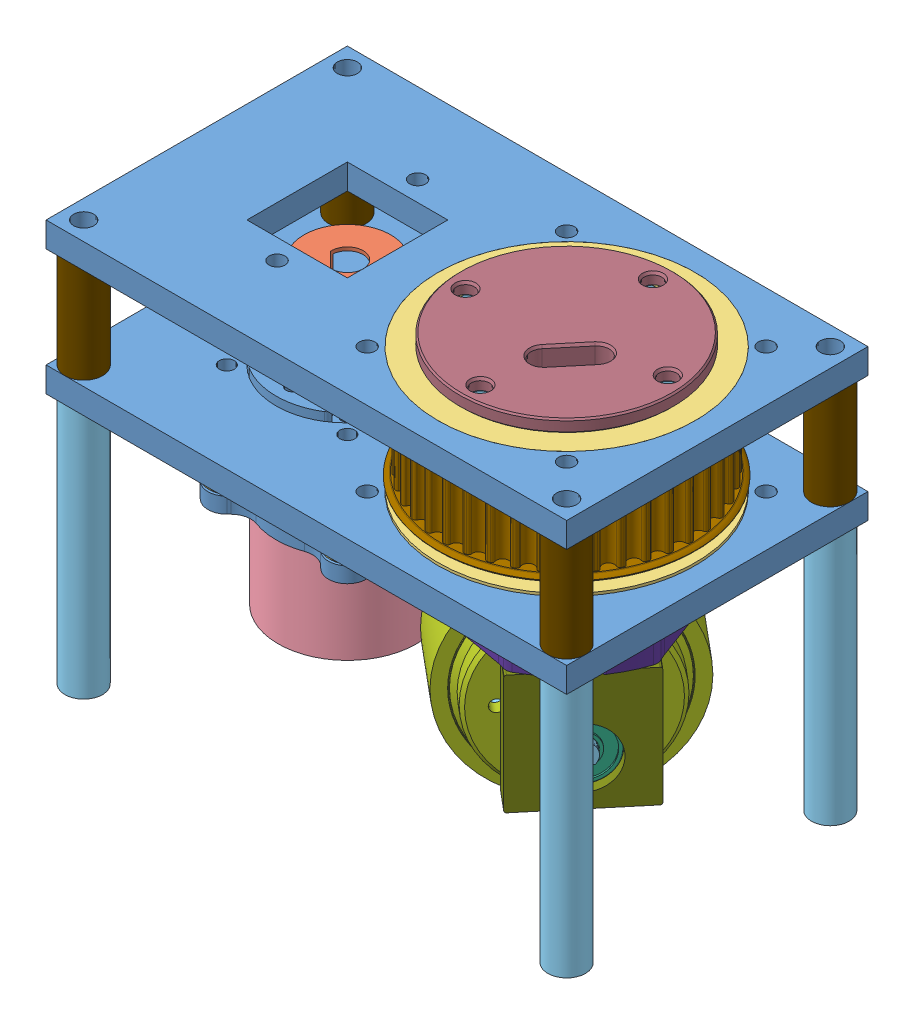
SolidWorks assembly Gearbox Wheel Prototype, configuration Default. Lengths in mm.
Overall size (151.59 104.78 115.16).
35 component instances, 23 part files, 32 mates.
Components (placement in the parent):
- Gearbox Wheel Prototype Structure-1: Gearbox Wheel Prototype Structure [Default] at origin size (131.66 38.1 76.2)
- Manufacture Ready Swerve_Double Gearbox Wheel_Assem-1: Manufacture Ready Swerve_Double Gearbox Wheel_Assem [Default] at (0 -47.625 0) x (0.76734 0 0.64124) z (-0.64124 0 0.76734) size (84.23 95.25 79.69)
  - PROPDRIVE 2836-1: PROPDRIVE 2836 [Default] at (-7.34 47.9628 0) x (0 0.80165 -0.597794) z (0 0.597794 0.80165) size (28 45.1 28)
  - Zoro Bearing 50mmID 65mm OD 7mmWidth-1: Zoro Bearing 50mmID 65mm OD 7mmWidth [Default] at (0 63.175 0) x (0.965482 0 -0.260469) z (0.260469 0 0.965482) size (65 7 65)
  - Zoro Bearing 50mmID 65mm OD 7mmWidth-2: Zoro Bearing 50mmID 65mm OD 7mmWidth [Default] at (0 32.075 0) x (0.000165 0 -1) z (1 0 0.000165) size (65 7 65)
  - Propdrive Shaft Pully-1: Propdrive Shaft Pully [Default] at (20.1995 47.9628 0) x (0 -0.036242 0.999343) z (0 -0.999343 -0.036242) size (15.88 9.14 15.88)
  - Double Gearbox 36mm 19 to 1-2: Double Gearbox 36mm 19 to 1 [Default] at (-5.8885 0 0) x (0 0 1) z (0 1 0) size (36 77 36)
  - FL696ZZ-1: FL696ZZ [Default] at (30.7875 0 0) x (-1 0 0) z (0 -0.99717 0.07518) size (5 17 17)
  - Casted Swerve Wheel-1: Casted Swerve Wheel [Default] at (0.0588 0 0) size (25.93 50.8 50.8)
  - Custom Input Shaft Pully-1: Custom Input Shaft Pully [Default] at (20.1995 0 0) x (0 0 1) z (0 1 0) size (21.89 11.18 21.89)
  - 5mm Pully Interface-1: 5mm Pully Interface [Default] at origin size (65.57 21.67 65.57)
  - Bottom Bearing Retainer-1: Bottom Bearing Retainer [Default] at origin size (56.35 4.76 56.35)
  - Drive Motor Face Mount-1: Drive Motor Face Mount [Default] at origin size (2.29 30.23 43.18)
  - Gearbox-Side Support-1: Gearbox-Side Support [Default] at origin size (6.35 34.92 28.57)
  - Inner Modual Lid-1: Inner Modual Lid [Default] at origin size (53.98 6.35 53.98)
  - Innermost Structure-1: Innermost Structure [Default] at origin size (51.14 38.65 53.98)
  - Left Motor Mount Retainer-1: Left Motor Mount Retainer [Default] at origin size (13.3 15.88 8.58)
  - Pully-Side Support-1: Pully-Side Support [Default] at origin size (6.35 34.92 28.57)
  - Wheel Support Mount Plate-1: Wheel Support Mount Plate [Default] at origin size (69.4 4.76 56.35)
  - Left Motor Mount Retainer-2: Left Motor Mount Retainer [Right] at origin size (13.3 16.31 8.58)
- RB Standoff_-1: RB Standoff_ [1000L] at (33.3375 0 33.3375) size (9.53 25.4 9.53)
- RB Standoff_-3: RB Standoff_ [1000L] at (-88.7984 0 -33.3375) x (0.918365 0 -0.395734) z (0.395734 0 0.918365) size (9.53 25.4 9.53)
- RB Standoff_-4: RB Standoff_ [1000L] at (-88.7984 0 33.3375) x (0.8 0 -0.6) z (0.6 0 0.8) size (9.53 25.4 9.53)
- RB Standoff_-5: RB Standoff_ [1000L] at (33.3375 0 -33.3375) x (0.63358 0 -0.773678) z (0.773678 0 0.63358) size (9.53 25.4 9.53)
- 36mm 34.7 (19_1, 27_1) gear box -1: 36mm 34.7 (19_1, 27_1) gear box  [Default] at (-55.4609 -38.1 0) x (-0.707107 0 -0.707107) z (0.707107 0 -0.707107) size (52.63 51.5 52.63)
- Swerve Turn Pinion 5mm HTD Pulley-1: Swerve Turn Pinion 5mm HTD Pulley [RBP-5245] at (-55.4609 1.1265 0) x (0.707107 0 0.707107) z (-0.707107 0 0.707107) size (21.89 18.41 21.89)
- Proto Gearbox Spacer-1: Proto Gearbox Spacer [Default] at (-70.7009 -28.575 -15.24) x (0.707107 0 0.707107) z (-0.707107 0 0.707107) size (8.16 19.05 9.53)
- Proto Gearbox Spacer-2: Proto Gearbox Spacer [Default] at (-70.7009 -28.575 15.24) x (0.707107 0 -0.707107) z (0.707107 0 0.707107) size (8.16 19.05 9.53)
- Proto Gearbox Spacer-3: Proto Gearbox Spacer [Default] at (-40.2209 -28.575 15.24) x (-0.707107 0 -0.707107) z (0.707107 0 -0.707107) size (8.16 19.05 9.53)
- Proto Gearbox Spacer-4: Proto Gearbox Spacer [Default] at (-40.2209 -28.575 -15.24) x (-0.707107 0 0.707107) z (-0.707107 0 -0.707107) size (8.16 19.05 9.53)
- COBRA 2808_22-1: COBRA 2808_22 [Default] at (-55.4609 -56.087 0) x (-0.837169 0 -0.546944) z (-0.546944 0 0.837169) size (35 45.1 35)
- RB Spacer_-2: RB Spacer_ [2500L] at (-88.7984 -50.8 33.3375) x (0.997425 0 0.071717) z (-0.071717 0 0.997425) size (9.53 63.5 9.53)
- RB Spacer_-3: RB Spacer_ [2500L] at (-88.7984 -50.8 -33.3375) x (0.993068 0 -0.117538) z (0.117538 0 0.993068) size (9.53 63.5 9.53)
- RB Spacer_-4: RB Spacer_ [2500L] at (33.3375 -50.8 33.3375) x (0.944381 0 -0.328853) z (0.328853 0 0.944381) size (9.53 63.5 9.53)
- RB Spacer_-5: RB Spacer_ [2500L] at (33.3375 -50.8 -33.3375) x (0.84097 0 -0.541082) z (0.541082 0 0.84097) size (9.53 63.5 9.53)
Mates (geometry in assembly coordinates):
- Coincident1: coincident aligned: plane of Gearbox Wheel Prototype Structure-1 through (0 0 0) normal (0 0 1)
- Coincident2: coincident aligned: plane of Gearbox Wheel Prototype Structure-1 through (0 0 0) normal (0 1 0)
- Coincident3: coincident aligned: plane of Gearbox Wheel Prototype Structure-1 through (0 0 0) normal (1 0 0)
- Coincident4: coincident aligned: plane of Gearbox Wheel Prototype Structure-1 through (0 19.05 0) normal (0 1 0); plane of Manufacture Ready Swerve_Double Gearbox Wheel_Assem-1/Zoro Bearing 50mmID 65mm OD 7mmWidth-1 through (0 19.05 0) normal (0 1 0)
- Concentric1: concentric anti-aligned: cylinder of Gearbox Wheel Prototype Structure-1 through (0 12.7 0) axis (0 1 0) radius 32.5; cylinder of Manufacture Ready Swerve_Double Gearbox Wheel_Assem-1/Zoro Bearing 50mmID 65mm OD 7mmWidth-1 through (0 19.05 0) axis (0 -1 0) radius 32.5
- Concentric2: concentric anti-aligned: cylinder of Gearbox Wheel Prototype Structure-1 through (33.3375 -19.05 33.3375) axis (0 1 0) radius 2.5527; cylinder of RB Standoff_-1 through (33.3375 12.7 33.3375) axis (0 -1 0) radius 4.7625
- Coincident5: coincident anti-aligned: plane of Gearbox Wheel Prototype Structure-1 through (0 12.7 0) normal (0 -1 0); plane of RB Standoff_-1 through (33.3375 12.7 33.3375) normal (0 1 0)
- Coincident7: coincident anti-aligned: plane of Gearbox Wheel Prototype Structure-1 through (0 12.7 0) normal (0 -1 0); plane of RB Standoff_-3 through (-88.7984 12.7 -33.3375) normal (0 1 0)
- Coincident8: coincident anti-aligned: plane of Gearbox Wheel Prototype Structure-1 through (0 12.7 0) normal (0 -1 0); plane of RB Standoff_-4 through (-88.7984 12.7 33.3375) normal (0 1 0)
- Coincident9: coincident anti-aligned: plane of Gearbox Wheel Prototype Structure-1 through (0 12.7 0) normal (0 -1 0); plane of RB Standoff_-5 through (33.3375 12.7 -33.3375) normal (0 1 0)
- Concentric3: concentric anti-aligned: cylinder of Gearbox Wheel Prototype Structure-1 through (33.3375 -19.05 -33.3375) axis (0 1 0) radius 2.5527; cylinder of RB Standoff_-5 through (33.3375 12.7 -33.3375) axis (0 -1 0) radius 4.7625
- Concentric4: concentric anti-aligned: cylinder of Gearbox Wheel Prototype Structure-1 through (-88.7984 -19.05 33.3375) axis (0 1 0) radius 2.5527; cylinder of RB Standoff_-4 through (-88.7984 12.7 33.3375) axis (0 -1 0) radius 4.7625
- Concentric5: concentric anti-aligned: cylinder of Gearbox Wheel Prototype Structure-1 through (-88.7984 -19.05 -33.3375) axis (0 1 0) radius 2.5527; cylinder of RB Standoff_-3 through (-88.7984 12.7 -33.3375) axis (0 -1 0) radius 4.7625
- Concentric6: concentric anti-aligned: cylinder of 36mm 34.7 (19_1, 27_1) gear box -1 through (-55.4609 -10.541 0) axis (0 1 0) radius 4; cylinder of Swerve Turn Pinion 5mm HTD Pulley-1 through (-55.4609 10.334 0) axis (0 -1 0) radius 4
- Parallel1: parallel anti-aligned: plane of 36mm 34.7 (19_1, 27_1) gear box -1 through (-59.4419 9.459 -0.3889) normal (-0.707107 0 0.707107); plane of Swerve Turn Pinion 5mm HTD Pulley-1 through (-59.453 10.334 0.2505) normal (0.707107 0 -0.707107)
- Coincident12: coincident anti-aligned: plane of 36mm 34.7 (19_1, 27_1) gear box -1 through (-57.7731 -5.541 2.3122) normal (0 1 0); plane of Swerve Turn Pinion 5mm HTD Pulley-1 through (-55.4609 -5.541 0) normal (0 -1 0)
- Concentric7: concentric anti-aligned: cylinder of Gearbox Wheel Prototype Structure-1 through (-55.4609 19.051 0) axis (0 -1 0) radius 18; cylinder of 36mm 34.7 (19_1, 27_1) gear box -1 through (-55.4609 -38.1 0) axis (0 1 0) radius 18
- Concentric8: concentric anti-aligned: cylinder of Gearbox Wheel Prototype Structure-1 through (-70.7009 19.051 15.24) axis (0 -1 0) radius 1.905; cylinder of 36mm 34.7 (19_1, 27_1) gear box -1 through (-70.7009 -42.672 15.24) axis (0 1 0) radius 1.3843
- Concentric10: concentric anti-aligned: cylinder of 36mm 34.7 (19_1, 27_1) gear box -1 through (-70.7009 -42.672 -15.24) axis (0 1 0) radius 1.3843; cylinder of Proto Gearbox Spacer-1 through (-70.7009 -19.05 -15.24) axis (0 -1 0) radius 1.905
- Coincident13: coincident anti-aligned: plane of Gearbox Wheel Prototype Structure-1 through (0 -19.05 0) normal (0 -1 0); plane of Proto Gearbox Spacer-1 through (-63.0809 -19.05 -7.62) normal (0 1 0)
- Coincident14: coincident anti-aligned: plane of 36mm 34.7 (19_1, 27_1) gear box -1 through (-55.4609 -38.1 0) normal (0 1 0); plane of Proto Gearbox Spacer-1 through (-63.0809 -38.1 -7.62) normal (0 -1 0)
- Concentric11: concentric anti-aligned: cylinder of 36mm 34.7 (19_1, 27_1) gear box -1 through (-55.4609 -38.1 0) axis (0 1 0) radius 18; cylinder of Proto Gearbox Spacer-1 through (-55.4609 -19.05 0) axis (0 -1 0) radius 18.254
- Concentric12: concentric aligned: cylinder of 36mm 34.7 (19_1, 27_1) gear box -1 through (-55.4609 -35.687 0) axis (0 -1 0) radius 4; cylinder of COBRA 2808_22-1 through (-55.4609 24.5531 0) axis (0 -1 0) radius 1.5875
- Coincident15: coincident anti-aligned: plane of 36mm 34.7 (19_1, 27_1) gear box -1 through (-55.4609 -42.037 0) normal (0 -1 0); plane of COBRA 2808_22-1 through (-55.4609 -42.037 0) normal (0 1 0)
- Concentric13: concentric anti-aligned: cylinder of Gearbox Wheel Prototype Structure-1 through (-88.7984 -19.05 33.3375) axis (0 1 0) radius 2.5527; cylinder of RB Spacer_-2 through (-88.7984 -19.05 33.3375) axis (0 -1 0) radius 4.7625
- Coincident16: coincident anti-aligned: plane of Gearbox Wheel Prototype Structure-1 through (0 -19.05 0) normal (0 -1 0); plane of RB Spacer_-2 through (-88.7984 -19.05 33.3375) normal (0 1 0)
- Coincident17: coincident: plane of Gearbox Wheel Prototype Structure-1 through (0 -19.05 0) normal (0 -1 0); plane of RB Spacer_-3 through (-80.5851 -19.05 51.4671) normal (0 1 0)
- Coincident18: coincident: plane of Gearbox Wheel Prototype Structure-1 through (0 -19.05 0) normal (0 -1 0); plane of RB Spacer_-4 through (-70.1126 -19.05 68.9418) normal (0 1 0)
- Coincident19: coincident: plane of Gearbox Wheel Prototype Structure-1 through (0 -19.05 0) normal (0 -1 0); plane of RB Spacer_-5 through (-57.5725 -19.05 85.1857) normal (0 1 0)
- Concentric14: concentric anti-aligned: cylinder of Gearbox Wheel Prototype Structure-1 through (-88.7984 -19.05 -33.3375) axis (0 1 0) radius 2.5527; cylinder of RB Spacer_-3 through (-88.7984 -19.05 -33.3375) axis (0 -1 0) radius 4.7625
- Concentric15: concentric anti-aligned: cylinder of Gearbox Wheel Prototype Structure-1 through (33.3375 -19.05 33.3375) axis (0 1 0) radius 2.5527; cylinder of RB Spacer_-4 through (33.3375 -19.05 33.3375) axis (0 -1 0) radius 4.7625
- Concentric16: concentric anti-aligned: cylinder of Gearbox Wheel Prototype Structure-1 through (33.3375 -19.05 -33.3375) axis (0 1 0) radius 2.5527; cylinder of RB Spacer_-5 through (33.3375 -19.05 -33.3375) axis (0 -1 0) radius 4.7625
